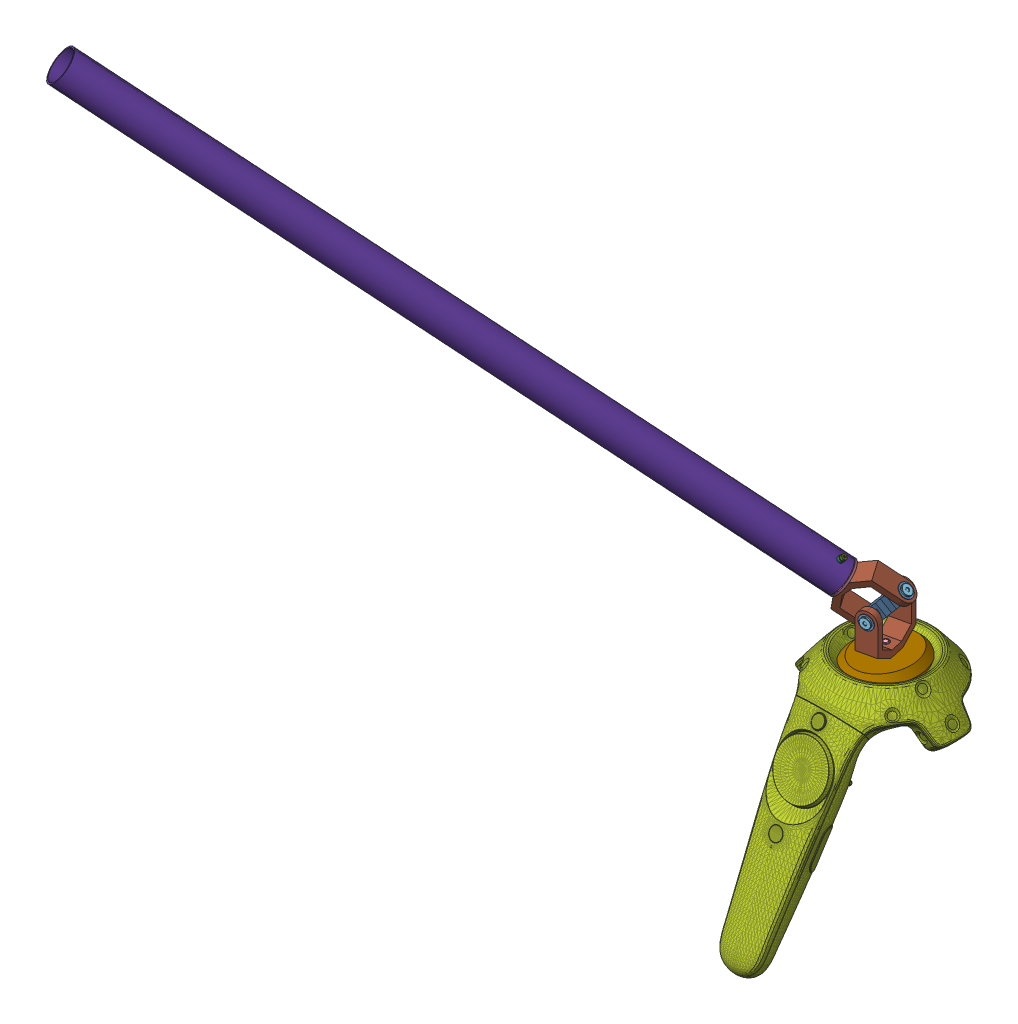
SolidWorks assembly WandMountC, configuration Default. Lengths in mm.
Overall size (407.06 600.86 382.33).
39 component instances, 17 part files, 83 mates.
Components (placement in the parent):
- 57155K301_Stainless Steel Ball BearingB-5: 57155K301_Stainless Steel Ball BearingB [57155K301] at (0 1.0795 0) x (-0.199974 0 0.979801) z (0 1 0) size (10.72 10.72 3.17)
- 57155K301_Stainless Steel Ball BearingB-6: 57155K301_Stainless Steel Ball BearingB [57155K301] at (0 13.9205 0) x (0.455162 0 -0.890409) z (0 -1 0) size (10.72 10.72 3.17)
- 94459A310_Heat-Set Inserts for PlasticB-1: 94459A310_Heat-Set Inserts for PlasticB [94459A310] at (0 4.699 -12.5) x (0.43803 0 0.898961) z (0.898961 0 -0.43803) size (6.45 5.21 6.45)
- 94459A310_Heat-Set Inserts for PlasticB-2: 94459A310_Heat-Set Inserts for PlasticB [94459A310] at (0 4.699 12.5) x (0.130741 0 -0.991417) z (-0.991417 0 -0.130741) size (6.45 5.21 6.45)
- 91251A196_Black-Oxide Alloy Steel Socket Head Screw-1: 91251A196_Black-Oxide Alloy Steel Socket Head Screw [91251A196] at (0 -5.6453 12.5) x (0.587183 0 -0.809454) z (0 -1 0) size (6.86 6.86 20.6)
- 91251A196_Black-Oxide Alloy Steel Socket Head Screw-2: 91251A196_Black-Oxide Alloy Steel Socket Head Screw [91251A196] at (0 -5.6453 -12.5) x (0.424116 0 -0.905608) z (0 -1 0) size (6.86 6.86 20.6)
- 92012A207_Alloy Steel Precision Shoulder Screw-1: 92012A207_Alloy Steel Precision Shoulder Screw [92012A207] at (0 -6.0643 0) x (-0.696496 0 0.717561) z (0 -1 0) size (7.94 7.94 28.23)
- 94459A310_Heat-Set Inserts for PlasticB-10: 94459A310_Heat-Set Inserts for PlasticB [94459A310] at (-1.165 46.3018 -5.1714) x (-0.720131 0.674604 0.162234) z (-0.658111 -0.738179 0.148262) size (6.45 5.21 6.45)
- 94459A310_Heat-Set Inserts for PlasticB-11: 94459A310_Heat-Set Inserts for PlasticB [94459A310] at (-3.4886 42.3887 0.7859) x (-0.75187 0.633921 -0.181208) z (-0.039778 0.230728 0.972205) size (6.45 5.21 6.45)
- 94459A310_Heat-Set Inserts for PlasticB-12: 94459A310_Heat-Set Inserts for PlasticB [94459A310] at (1.165 46.3018 5.1714) x (0.372122 0.92439 -0.083833) z (0.901789 -0.381449 -0.203159) size (6.45 5.21 6.45)
- 94459A310_Heat-Set Inserts for PlasticB-13: 94459A310_Heat-Set Inserts for PlasticB [94459A310] at (3.4886 50.2148 -0.7859) x (-0.720131 0.674604 0.162234) z (-0.219776 0 -0.97555) size (6.45 5.21 6.45)
- 57155K301_Stainless Steel Ball BearingB-7: 57155K301_Stainless Steel Ball BearingB [57155K301] at (4.1583 46.3018 18.4579) x (0.349901 -0.933464 -0.078827) z (-0.219776 0 -0.97555) size (10.72 10.72 3.17)
- 57155K301_Stainless Steel Ball BearingB-8: 57155K301_Stainless Steel Ball BearingB [57155K301] at (-12.4518 32.335 2.8052) x (0.134477 -0.308991 -0.94151) z (0.658111 0.738179 -0.148262) size (10.72 10.72 3.17)
- 57155K301_Stainless Steel Ball BearingB-9: 57155K301_Stainless Steel Ball BearingB [57155K301] at (-4.1583 46.3018 -18.4579) x (0.958856 -0.184207 -0.216015) z (0.219776 0 0.97555) size (10.72 10.72 3.17)
- 57155K301_Stainless Steel Ball BearingB-10: 57155K301_Stainless Steel Ball BearingB [57155K301] at (12.4518 60.2685 -2.8052) x (0.557619 -0.345544 0.754759) z (-0.658111 -0.738179 0.148262) size (10.72 10.72 3.17)
- 90318A302_Ultra-Low-Profile Precision Shoulder Screw-1: 90318A302_Ultra-Low-Profile Precision Shoulder Screw [90318A302] at (-4.7688 46.3018 -21.1681) x (0.151242 0.987909 -0.034072) z (-0.219776 0 -0.97555) size (7.94 7.94 15.93)
- 90318A302_Ultra-Low-Profile Precision Shoulder Screw-2: 90318A302_Ultra-Low-Profile Precision Shoulder Screw [90318A302] at (-14.2801 30.2843 3.2171) x (-0.381869 0.157538 -0.910691) z (-0.658111 -0.738179 0.148262) size (7.94 7.94 15.93)
- 90318A302_Ultra-Low-Profile Precision Shoulder Screw-3: 90318A302_Ultra-Low-Profile Precision Shoulder Screw [90318A302] at (4.7688 46.3018 21.1681) x (-0.546533 0.828337 0.123125) z (0.219776 0 0.97555) size (7.94 7.94 15.93)
- 90318A302_Ultra-Low-Profile Precision Shoulder Screw-4: 90318A302_Ultra-Low-Profile Precision Shoulder Screw [90318A302] at (14.2801 62.3192 -3.2171) x (-0.21426 0.372386 0.903007) z (0.658111 0.738179 -0.148262) size (7.94 7.94 15.93)
- 94459A310_Heat-Set Inserts for PlasticB-15: 94459A310_Heat-Set Inserts for PlasticB [94459A310] at (0 21.0008 0) x (0.601643 0 0.798765) z (0.798765 0 -0.601643) size (6.45 5.21 6.45)
- 90357A127_Ultra-Low-Profile Socket Head Screw-1: 90357A127_Ultra-Low-Profile Socket Head Screw [90357A127] at (-13.3303 60.7381 12.7062) x (0.818605 0.484769 0.308033) z (-0.569674 0.616944 0.543003) size (8.46 8.46 11.46)
- 94459A310_Heat-Set Inserts for PlasticB-16: 94459A310_Heat-Set Inserts for PlasticB [94459A310] at (-19.7671 67.7091 18.8417) x (-0.81731 -0.494767 -0.295315) z (0.086467 -0.612035 0.78609) size (6.45 5.21 6.45)
- Vive Controller 1.5B-1: Vive Controller 1.5B [Default] at (0.0016 6.0546 36.5874) x (1 -0.000227 0) z (-0.000192 -0.847056 0.531504) size (118.44 84.37 219.45)
- BottomPlugB-2: BottomPlugB [Default] at origin size (42.24 11.38 42.24)
- TopPlugB-2: TopPlugB [Default] at origin size (50.17 16.12 56.99)
- Cross-1: Cross [Default] at (0 46.3018 0) x (-0.219776 0 -0.97555) z (-0.658111 -0.738179 0.148262) size (20 10 20)
- FORK-1: FORK [Default] at (0 46.3018 0) x (-0.219776 0 -0.97555) z (0 1 0) size (40 15 37.5)
- FORK-2: FORK [Default] at (0 46.3018 0) x (-0.658111 -0.738179 0.148262) z (0.569674 -0.616944 -0.543003) size (40 15 37.5)
- GimbalSpacerP3B-9: GimbalSpacerP3B [Default] at (0 -1.3017 0) x (0 1 0) z (0.558736 0 0.829346) size (0.79 8 8)
- GimbalSpacerP3B-10: GimbalSpacerP3B [Default] at (0 -2.0955 0) x (0 1 0) z (0.705019 0 0.709189) size (0.79 8 8)
- GimbalSpacerP3B-11: GimbalSpacerP3B [Default] at (0 15.508 0) x (0 1 0) z (0.841324 0 0.540531) size (0.79 8 8)
- GimbalPlugP3C-1: GimbalPlugP3C [Default] at (-17.0902 64.8101 16.2901) x (0.692842 0.715883 -0.086493) z (0.442088 -0.326943 0.835265) size (25.4 16.5 25.4)
- 94459A418_Heat-Set Inserts for PlasticP3B-1: 94459A418_Heat-Set Inserts for PlasticP3B [94459A418] at (-28.2294 66.5917 22.8832) x (0.619885 -0.530023 0.578635) z (0.368392 -0.454518 -0.810987) size (3.8 4.42 3.8)
- ClampSpacer-1: ClampSpacer [Default] at (-32.0308 62.664 23.3578) x (-0.692842 -0.715883 0.086493) z (0.442088 -0.326943 0.835265) size (2.63 4.5 4.5)
- 91290A015_Black-Oxide Alloy Steel Socket Head Screw-1: 91290A015_Black-Oxide Alloy Steel Socket Head Screw [91290A015] at (-31.6844 63.0219 23.3145) x (0.116559 0.007185 0.993158) z (-0.692842 -0.715883 0.086493) size (3.8 3.8 10.09)
- 94459A418_Heat-Set Inserts for PlasticP3B-2: 94459A418_Heat-Set Inserts for PlasticP3B [94459A418] at (-18.5123 76.632 21.6702) x (0.573911 -0.620068 -0.534923) z (0.436574 -0.320978 0.840462) size (3.8 4.42 3.8)
- 91290A015_Black-Oxide Alloy Steel Socket Head Screw-2: 91290A015_Black-Oxide Alloy Steel Socket Head Screw [91290A015] at (-15.0574 80.2018 21.2389) x (0.266503 -0.14276 0.953203) z (0.692842 0.715883 -0.086493) size (3.8 3.8 10.09)
- ClampSpacer-3: ClampSpacer [Default] at (-14.711 80.5598 21.1956) x (0.692842 0.715883 -0.086493) z (-0.442088 0.326943 -0.835265) size (2.63 4.5 4.5)
- MainTubeP3-1: MainTubeP3 [Default] at (-18.2438 66.0594 17.3897) x (-0.692842 -0.715883 0.086493) z (-0.569674 0.616944 0.543003) size (25.4 25.4 553.63)
Mates (geometry in assembly coordinates):
- Coincident5: coincident aligned: plane of Vive Controller 1.5-1 through (0.0016 0 36.5874) normal (0 1 0)
- Coincident4: coordinate: point of BottomPlug-2
- Coincident6: coincident: line of Vive Controller 1.5-1 through (0 0 0) axis (0 1 0)
- Coincident7: coincident: line of Vive Controller 1.5-1 through (0 0 0) axis (0 1 0)
- Parallel1: parallel anti-aligned: plane of Vive Controller 1.5-1 through (0.0016 6.0546 -0.0032) normal (0 0 -1)
- Coincident9: coordinate: unknown of TopPlugB-2
- Concentric3: concentric anti-aligned: cylinder of BottomPlugB-2 through (0 -11.5 -12.5) axis (0 -1 0) radius 2.2479; cylinder of 94459A310_Heat-Set Inserts for PlasticB-1 through (0 4.699 -12.5) axis (0 1 0) radius 2.7686
- Concentric4: concentric anti-aligned: cylinder of BottomPlugB-2 through (0 -11.5 12.5) axis (0 -1 0) radius 2.2479; cylinder of 94459A310_Heat-Set Inserts for PlasticB-2 through (0 4.699 12.5) axis (0 1 0) radius 2.7686
- Concentric45: concentric aligned: cylinder of 57155K301_Stainless Steel Ball BearingB-5 through (0 1.0795 0) axis (0 1 0) radius 2.3813; cylinder of 92012A207_Alloy Steel Precision Shoulder Screw-1 through (0 21.717 0) axis (0 1 0) radius 2.3813
- Concentric47: concentric anti-aligned: cylinder of 57155K301_Stainless Steel Ball BearingB-6 through (0 13.9205 0) axis (0 -1 0) radius 2.3813; cylinder of 92012A207_Alloy Steel Precision Shoulder Screw-1 through (0 21.717 0) axis (0 1 0) radius 2.3813
- Coincident39: coincident aligned: plane of TopPlugB-2 through (0 0 0) normal (0 -1 0); plane of 94459A310_Heat-Set Inserts for PlasticB-2 through (0.4134 0 9.3648) normal (0 -1 0)
- Concentric54: concentric anti-aligned: cylinder of TopPlugB-2 through (0 5.5 -12.5) axis (0 -1 0) radius 2.8067; cylinder of 94459A310_Heat-Set Inserts for PlasticB-1 through (0 4.699 -12.5) axis (0 1 0) radius 2.7686
- Coincident40: coincident aligned: plane of TopPlugB-2 through (0 0 0) normal (0 -1 0); plane of 94459A310_Heat-Set Inserts for PlasticB-1 through (1.3852 0 -9.6572) normal (0 -1 0)
- Concentric55: concentric anti-aligned: cylinder of TopPlugB-2 through (0 5.5 12.5) axis (0 -1 0) radius 2.8067; cylinder of 94459A310_Heat-Set Inserts for PlasticB-2 through (0 4.699 12.5) axis (0 1 0) radius 2.7686
- Concentric56: concentric anti-aligned: cylinder of TopPlugB-2 through (0 3.5 0) axis (0 -1 0) radius 4.7625; cylinder of 57155K301_Stainless Steel Ball BearingB-5 through (0 1.0795 0) axis (0 1 0) radius 4.7625
- Coincident41: coincident anti-aligned: plane of TopPlugB-2 through (0 0 0) normal (0 -1 0); plane of 57155K301_Stainless Steel Ball BearingB-5 through (5.2511 0 1.0717) normal (0 1 0)
- Concentric57: concentric anti-aligned: cylinder of TopPlugB-2 through (0 11.5 0) axis (0 1 0) radius 4.7625; cylinder of 57155K301_Stainless Steel Ball BearingB-6 through (0 13.9205 0) axis (0 -1 0) radius 4.7625
- Coincident42: coincident anti-aligned: plane of TopPlugB-2 through (0 15 0) normal (0 1 0); plane of 57155K301_Stainless Steel Ball BearingB-6 through (4.7721 15 2.4394) normal (0 -1 0)
- Concentric63: concentric anti-aligned: cylinder of BottomPlugB-2 through (0 -11.5 12.5) axis (0 -1 0) radius 2.2479; cylinder of 91251A196_Black-Oxide Alloy Steel Socket Head Screw-1 through (0 4.375 12.5) axis (0 1 0) radius 3.429
- Coincident43: coincident anti-aligned: plane of BottomPlugB-2 through (0 -11.5 0) normal (0 -1 0); plane of 91251A196_Black-Oxide Alloy Steel Socket Head Screw-1 through (2.4384 -11.5 14.2689) normal (0 1 0)
- Concentric64: concentric anti-aligned: cylinder of BottomPlugB-2 through (0 -11.5 -12.5) axis (0 -1 0) radius 2.2479; cylinder of 91251A196_Black-Oxide Alloy Steel Socket Head Screw-2 through (0 4.375 -12.5) axis (0 1 0) radius 3.429
- Coincident44: coincident anti-aligned: plane of BottomPlugB-2 through (0 -11.5 0) normal (0 -1 0); plane of 91251A196_Black-Oxide Alloy Steel Socket Head Screw-2 through (2.7281 -11.5 -11.2224) normal (0 1 0)
- Width1: width aligned: plane of FORK-1 through (-10.6133 53.8018 -12.9849) normal (0.219776 0 0.97555); plane of FORK-1 through (-4.02 27.0753 16.2816) normal (-0.219776 0 -0.97555); plane of Cross-1 through (5.7984 42.9287 8.9443) normal (0.219776 0 0.97555); plane of Cross-1 through (1.4029 42.9287 -10.5667) normal (-0.219776 0 -0.97555)
- Width2: width aligned: plane of FORK-2 through (-4.7734 71.2828 2.0171) normal (-0.658111 -0.738179 0.148262); plane of FORK-2 through (-9.2914 32.6487 -8.0476) normal (0.658111 0.738179 -0.148262); plane of Cross-1 through (-2.9805 35.5469 0.6714) normal (-0.658111 -0.738179 0.148262); plane of Cross-1 through (10.1818 50.3105 -2.2938) normal (0.658111 0.738179 -0.148262)
- Concentric65: concentric anti-aligned: cylinder of Cross-1 through (-1.0989 46.3018 -4.8778) axis (-0.219776 0 -0.97555) radius 2.8067; cylinder of 94459A310_Heat-Set Inserts for PlasticB-10 through (-1.165 46.3018 -5.1714) axis (0.219776 0 0.97555) radius 2.7686
- Coincident45: coincident aligned: plane of Cross-1 through (1.4029 42.9287 -10.5667) normal (-0.219776 0 -0.97555); plane of 94459A310_Heat-Set Inserts for PlasticB-10 through (-4.475 48.4351 -9.2425) normal (-0.219776 0 -0.97555)
- Concentric66: concentric anti-aligned: cylinder of Cross-1 through (-3.2906 42.6109 0.7413) axis (-0.658111 -0.738179 0.148262) radius 2.8067; cylinder of 94459A310_Heat-Set Inserts for PlasticB-11 through (-3.4886 42.3887 0.7859) axis (0.658111 0.738179 -0.148262) radius 2.7686
- Coincident46: coincident aligned: plane of Cross-1 through (-2.9805 35.5469 0.6714) normal (-0.658111 -0.738179 0.148262); plane of 94459A310_Heat-Set Inserts for PlasticB-11 through (-8.9587 40.9246 0.9096) normal (-0.658111 -0.738179 0.148262)
- Concentric5: concentric anti-aligned: cylinder of Cross-1 through (1.0989 46.3018 4.8778) axis (0.219776 0 0.97555) radius 2.8067; cylinder of 94459A310_Heat-Set Inserts for PlasticB-12 through (1.165 46.3018 5.1714) axis (-0.219776 0 -0.97555) radius 2.7686
- Coincident8: coincident aligned: plane of Cross-1 through (5.7984 42.9287 8.9443) normal (0.219776 0 0.97555); plane of 94459A310_Heat-Set Inserts for PlasticB-12 through (3.3745 49.2249 9.4904) normal (0.219776 0 0.97555)
- Concentric6: concentric anti-aligned: cylinder of Cross-1 through (3.2906 49.9926 -0.7413) axis (0.658111 0.738179 -0.148262) radius 2.8067; cylinder of 94459A310_Heat-Set Inserts for PlasticB-13 through (3.4886 50.2148 -0.7859) axis (-0.658111 -0.738179 0.148262) radius 2.7686
- Coincident47: coincident aligned: plane of Cross-1 through (10.1818 50.3105 -2.2938) normal (0.658111 0.738179 -0.148262); plane of 94459A310_Heat-Set Inserts for PlasticB-13 through (4.3038 55.8168 -0.9696) normal (0.658111 0.738179 -0.148262)
- Concentric7: concentric aligned: cylinder of FORK-1 through (4.3955 46.3018 19.511) axis (-0.219776 0 -0.97555) radius 4.7625; cylinder of 57155K301_Stainless Steel Ball BearingB-7 through (4.1583 46.3018 18.4579) axis (-0.219776 0 -0.97555) radius 4.7625
- Coincident10: coincident anti-aligned: plane of FORK-1 through (-2.9211 53.8018 21.1593) normal (0.219776 0 0.97555); plane of 57155K301_Stainless Steel Ball BearingB-7 through (-0.485 44.3795 20.6105) normal (-0.219776 0 -0.97555)
- Concentric9: concentric anti-aligned: cylinder of FORK-1 through (4.3955 46.3018 19.511) axis (-0.219776 0 -0.97555) radius 4.7625; cylinder of 57155K301_Stainless Steel Ball BearingB-9 through (-4.1583 46.3018 -18.4579) axis (0.219776 0 0.97555) radius 4.7625
- Coincident12: coincident anti-aligned: plane of FORK-1 through (-11.7121 24.2524 -17.8627) normal (-0.219776 0 -0.97555); plane of 57155K301_Stainless Steel Ball BearingB-9 through (-3.4324 51.5694 -19.728) normal (0.219776 0 0.97555)
- Concentric20: concentric aligned: cylinder of FORK-1 through (0 16.3018 0) axis (0 1 0) radius 2.8067; cylinder of 94459A310_Heat-Set Inserts for PlasticB-15 through (0 21.0008 0) axis (0 1 0) radius 2.7686
- Coincident19: coincident aligned: plane of FORK-1 through (-5.9476 16.3018 7.7252) normal (0 -1 0); plane of 94459A310_Heat-Set Inserts for PlasticB-15 through (1.9026 16.3018 2.5259) normal (0 -1 0)
- Concentric8: concentric anti-aligned: cylinder of FORK-2 through (13.1622 61.0653 -2.9652) axis (-0.658111 -0.738179 0.148262) radius 4.7625; cylinder of 57155K301_Stainless Steel Ball BearingB-8 through (-12.4518 32.335 2.8052) axis (0.658111 0.738179 -0.148262) radius 4.7625
- Coincident11: coincident anti-aligned: plane of FORK-2 through (-29.4154 47.1881 8.7391) normal (-0.658111 -0.738179 0.148262); plane of 57155K301_Stainless Steel Ball BearingB-8 through (-17.1325 34.7521 1.3434) normal (0.658111 0.738179 -0.148262)
- Concentric10: concentric aligned: cylinder of FORK-2 through (13.1622 61.0653 -2.9652) axis (-0.658111 -0.738179 0.148262) radius 4.7625; cylinder of 57155K301_Stainless Steel Ball BearingB-10 through (12.4518 60.2685 -2.8052) axis (-0.658111 -0.738179 0.148262) radius 4.7625
- Coincident13: coincident anti-aligned: plane of FORK-2 through (13.7425 58.485 -13.2368) normal (0.658111 0.738179 -0.148262); plane of 57155K301_Stainless Steel Ball BearingB-10 through (10.4508 64.1705 0.4596) normal (-0.658111 -0.738179 0.148262)
- Concentric12: concentric anti-aligned: circle of 94459A310_Heat-Set Inserts for PlasticB-10; cylinder of 90318A302_Ultra-Low-Profile Precision Shoulder Screw-1 through (-1.3671 46.3018 -6.0684) axis (0.219776 0 0.97555) radius 2.3813
- Concentric14: concentric anti-aligned: circle of 94459A310_Heat-Set Inserts for PlasticB-11; cylinder of 90318A302_Ultra-Low-Profile Precision Shoulder Screw-2 through (-4.0938 41.7099 0.9223) axis (0.658111 0.738179 -0.148262) radius 2.3813
- Concentric16: concentric anti-aligned: circle of 94459A310_Heat-Set Inserts for PlasticB-12; cylinder of 90318A302_Ultra-Low-Profile Precision Shoulder Screw-3 through (1.3671 46.3018 6.0684) axis (-0.219776 0 -0.97555) radius 2.3813
- Concentric18: concentric anti-aligned: circle of 94459A310_Heat-Set Inserts for PlasticB-13; cylinder of 90318A302_Ultra-Low-Profile Precision Shoulder Screw-4 through (4.0938 50.8936 -0.9223) axis (-0.658111 -0.738179 0.148262) radius 2.3813
- Concentric15: concentric aligned: cylinder of 57155K301_Stainless Steel Ball BearingB-7 through (4.1583 46.3018 18.4579) axis (-0.219776 0 -0.97555) radius 2.3813; cylinder of 90318A302_Ultra-Low-Profile Precision Shoulder Screw-3 through (1.3671 46.3018 6.0684) axis (-0.219776 0 -0.97555) radius 2.3813
- Coincident16: coincident anti-aligned: plane of 57155K301_Stainless Steel Ball BearingB-7 through (1.6882 45.1914 20.6417) normal (0.219776 0 0.97555); plane of 90318A302_Ultra-Low-Profile Precision Shoulder Screw-3 through (7.7142 48.5252 19.2841) normal (-0.219776 0 -0.97555)
- Concentric13: concentric aligned: cylinder of 57155K301_Stainless Steel Ball BearingB-8 through (-12.4518 32.335 2.8052) axis (0.658111 0.738179 -0.148262) radius 2.3813; cylinder of 90318A302_Ultra-Low-Profile Precision Shoulder Screw-2 through (-4.0938 41.7099 0.9223) axis (0.658111 0.738179 -0.148262) radius 2.3813
- Coincident15: coincident anti-aligned: plane of 57155K301_Stainless Steel Ball BearingB-8 through (-15.7898 33.0196 2.1038) normal (-0.658111 -0.738179 0.148262); plane of 90318A302_Ultra-Low-Profile Precision Shoulder Screw-2 through (-16.0718 33.7665 4.5708) normal (0.658111 0.738179 -0.148262)
- Concentric11: concentric aligned: cylinder of 57155K301_Stainless Steel Ball BearingB-9 through (-4.1583 46.3018 -18.4579) axis (0.219776 0 0.97555) radius 2.3813; cylinder of 90318A302_Ultra-Low-Profile Precision Shoulder Screw-1 through (-1.3671 46.3018 -6.0684) axis (0.219776 0 0.97555) radius 2.3813
- Coincident14: coincident anti-aligned: plane of 57155K301_Stainless Steel Ball BearingB-9 through (-3.9509 49.3444 -20.1319) normal (-0.219776 0 -0.97555); plane of 90318A302_Ultra-Low-Profile Precision Shoulder Screw-1 through (-8.3321 46.917 -19.1449) normal (0.219776 0 0.97555)
- Concentric17: concentric aligned: cylinder of 57155K301_Stainless Steel Ball BearingB-10 through (12.4518 60.2685 -2.8052) axis (-0.658111 -0.738179 0.148262) radius 2.3813; cylinder of 90318A302_Ultra-Low-Profile Precision Shoulder Screw-4 through (4.0938 50.8936 -0.9223) axis (-0.658111 -0.738179 0.148262) radius 2.3813
- Coincident17: coincident anti-aligned: plane of 57155K301_Stainless Steel Ball BearingB-10 through (11.9304 63.2339 -1.0624) normal (0.658111 0.738179 -0.148262); plane of 90318A302_Ultra-Low-Profile Precision Shoulder Screw-4 through (10.6319 63.6728 -4.6409) normal (-0.658111 -0.738179 0.148262)
- Concentric67: concentric aligned: cylinder of 92012A207_Alloy Steel Precision Shoulder Screw-1 through (0 21.717 0) axis (0 1 0) radius 2.3813; cylinder of 94459A310_Heat-Set Inserts for PlasticB-15 through (0 21.0008 0) axis (0 1 0) radius 2.7686
- Concentric68: concentric anti-aligned: cylinder of 92012A207_Alloy Steel Precision Shoulder Screw-1 through (0 21.717 0) axis (0 1 0) radius 2.3813; cylinder of GimbalSpacerP3B-9 through (0 -0.508 0) axis (0 -1 0) radius 2.3813
- Coincident48: coincident anti-aligned: plane of 57155K301_Stainless Steel Ball BearingB-5 through (3.0331 -0.508 0.619) normal (0 -1 0); plane of GimbalSpacerP3B-9 through (0 -0.508 0) normal (0 1 0)
- Concentric69: concentric anti-aligned: cylinder of 92012A207_Alloy Steel Precision Shoulder Screw-1 through (0 21.717 0) axis (0 1 0) radius 2.3813; cylinder of GimbalSpacerP3B-10 through (0 -1.3017 0) axis (0 -1 0) radius 2.3813
- Coincident49: coincident anti-aligned: plane of GimbalSpacerP3B-9 through (0 -1.3017 0) normal (0 -1 0); plane of GimbalSpacerP3B-10 through (0 -1.3017 0) normal (0 1 0)
- Concentric70: concentric anti-aligned: cylinder of 92012A207_Alloy Steel Precision Shoulder Screw-1 through (0 21.717 0) axis (0 1 0) radius 2.3813; cylinder of GimbalSpacerP3B-11 through (0 16.3018 0) axis (0 -1 0) radius 2.3813
- Coincident50: coincident anti-aligned: plane of 94459A310_Heat-Set Inserts for PlasticB-15 through (1.9026 16.3018 2.5259) normal (0 -1 0); plane of GimbalSpacerP3B-11 through (0 16.3018 0) normal (0 1 0)
- Coincident51: coincident anti-aligned: plane of 92012A207_Alloy Steel Precision Shoulder Screw-1 through (2.8478 -2.0955 2.7642) normal (0 1 0); plane of GimbalSpacerP3B-10 through (0 -2.0955 0) normal (0 -1 0)
- Coincident52: coincident anti-aligned: plane of 57155K301_Stainless Steel Ball BearingB-6 through (2.7564 15.508 1.409) normal (0 1 0); plane of GimbalSpacerP3B-11 through (0 15.508 0) normal (0 -1 0)
- Concentric72: concentric aligned: cylinder of FORK-2 through (-17.0902 64.8101 16.2901) axis (0.569674 -0.616944 -0.543003) radius 2.8067; cylinder of 90357A127_Ultra-Low-Profile Socket Head Screw-1 through (-14.2418 61.7253 13.5751) axis (0.569674 -0.616944 -0.543003) radius 4.2291
- Coincident54: coincident anti-aligned: plane of FORK-2 through (-21.2247 60.0812 8.1173) normal (0.569674 -0.616944 -0.543003); plane of 90357A127_Ultra-Low-Profile Socket Head Screw-1 through (-11.1261 63.5705 14.7475) normal (-0.569674 0.616944 0.543003)
- Concentric73: concentric anti-aligned: cylinder of GimbalPlugP3C-1 through (552.5837 -552.1335 -526.7129) axis (0.569674 -0.616944 -0.543003) radius 2.8067; cylinder of 94459A310_Heat-Set Inserts for PlasticB-16 through (-19.7671 67.7091 18.8417) axis (-0.569674 0.616944 0.543003) radius 2.7686
- Coincident55: coincident aligned: plane of GimbalPlugP3C-1 through (-11.4757 60.6579 26.8979) normal (0.569674 -0.616944 -0.543003); plane of 94459A310_Heat-Set Inserts for PlasticB-16 through (-19.6748 63.2455 15.3562) normal (0.569674 -0.616944 -0.543003)
- Concentric74: concentric aligned: cylinder of 90357A127_Ultra-Low-Profile Socket Head Screw-1 through (-14.2418 61.7253 13.5751) axis (0.569674 -0.616944 -0.543003) radius 4.2291; circle of 94459A310_Heat-Set Inserts for PlasticB-16
- Coincident56: coincident anti-aligned: plane of FORK-2 through (-16.683 71.455 9.1675) normal (-0.569674 0.616944 0.543003); plane of GimbalPlugP3C-1 through (-11.4757 60.6579 26.8979) normal (0.569674 -0.616944 -0.543003)
- Concentric75: concentric aligned: line of GimbalPlugP3C-1 through (-23.3709 71.6119 22.2767) axis (0.692842 0.715883 -0.086493); cylinder of 94459A418_Heat-Set Inserts for PlasticP3B-1 through (-28.2294 66.5917 22.8832) axis (0.692842 0.715883 -0.086493) radius 1.535
- Tangent1: tangent aligned: cylinder of GimbalPlugP3C-1 through (552.5837 -552.1335 -526.7129) axis (0.569674 -0.616944 -0.543003) radius 11.1125; plane of 94459A418_Heat-Set Inserts for PlasticP3B-1 through (-29.914 62.6681 24.317) normal (-0.692842 -0.715883 0.086493)
- Tangent3: tangent aligned: cylinder of GimbalPlugP3C-1 through (552.5837 -552.1335 -526.7129) axis (0.569674 -0.616944 -0.543003) radius 11.1125; plane of 94459A418_Heat-Set Inserts for PlasticP3B-2 through (-14.6013 78.4107 20.3179) normal (0.692842 0.715883 -0.086493)
- Concentric77: concentric anti-aligned: line of GimbalPlugP3C-1 through (-23.3709 71.6119 22.2767) axis (0.692842 0.715883 -0.086493); cylinder of 94459A418_Heat-Set Inserts for PlasticP3B-2 through (-18.5123 76.632 21.6702) axis (-0.692842 -0.715883 0.086493) radius 1.535
- Coincident57: coincident anti-aligned: axis of ClampSpacer-1 through (-33.7629 60.8743 23.574) axis (0.692842 0.715883 -0.086493); line of 94459A418_Heat-Set Inserts for PlasticP3B-2 through (-15.8711 79.361 21.3404) axis (-0.692842 -0.715883 0.086493)
- Concentric78: concentric aligned: cylinder of GimbalPlugP3C-1 through (552.5837 -552.1335 -526.7129) axis (0.569674 -0.616944 -0.543003) radius 11.1125; cylinder of ClampSpacer-1 through (-24.6526 73 23.4985) axis (0.569674 -0.616944 -0.543003) radius 12.7
- Concentric80: concentric aligned: line of 94459A418_Heat-Set Inserts for PlasticP3B-1 through (-31.0261 63.7021 23.2324) axis (0.692842 0.715883 -0.086493); cylinder of 91290A015_Black-Oxide Alloy Steel Socket Head Screw-1 through (-28.2201 66.6013 22.8821) axis (0.692842 0.715883 -0.086493) radius 1.9
- Coincident59: coincident anti-aligned: plane of ClampSpacer-1 through (-33.7629 60.8743 23.574) normal (-0.692842 -0.715883 0.086493); plane of 91290A015_Black-Oxide Alloy Steel Socket Head Screw-1 through (-35.0438 62.131 23.7152) normal (0.692842 0.715883 -0.086493)
- Coincident60: coincident anti-aligned: plane of 91290A015_Black-Oxide Alloy Steel Socket Head Screw-2 through (-11.7728 81.1192 20.4579) normal (-0.692842 -0.715883 0.086493); plane of ClampSpacer-3 through (-12.9789 82.3495 20.9794) normal (0.692842 0.715883 -0.086493)
- Coincident61: coincident aligned: line of 94459A418_Heat-Set Inserts for PlasticP3B-2 through (-15.7157 79.5217 21.321) axis (-0.692842 -0.715883 0.086493); line of ClampSpacer-3 through (-12.9789 82.3495 20.9794) axis (-0.692842 -0.715883 0.086493)
- Concentric81: concentric aligned: cylinder of GimbalPlugP3C-1 through (552.5837 -552.1335 -526.7129) axis (0.569674 -0.616944 -0.543003) radius 11.1125; cylinder of ClampSpacer-3 through (-24.6526 73 23.4985) axis (0.569674 -0.616944 -0.543003) radius 12.7
- Concentric82: concentric aligned: line of 94459A418_Heat-Set Inserts for PlasticP3B-2 through (-15.8711 79.361 21.3404) axis (-0.692842 -0.715883 0.086493); cylinder of 91290A015_Black-Oxide Alloy Steel Socket Head Screw-2 through (-18.5216 76.6224 21.6713) axis (-0.692842 -0.715883 0.086493) radius 1.9
- Coincident62: coincident aligned: line of 91290A015_Black-Oxide Alloy Steel Socket Head Screw-2 through (-12.9789 82.3495 20.9794) axis (-0.692842 -0.715883 0.086493); line of MainTubeP3-1 through (-14.5718 80.7036 21.1782) axis (-0.692842 -0.715883 0.086493)
- Coincident63: coincident aligned: line of GimbalPlugP3C-1 through (-26.4898 74.9896 25.2496) axis (0.569674 -0.616944 -0.543003); line of MainTubeP3-1 through (-333.6324 407.6179 318.0124) axis (0.569674 -0.616944 -0.543003)
